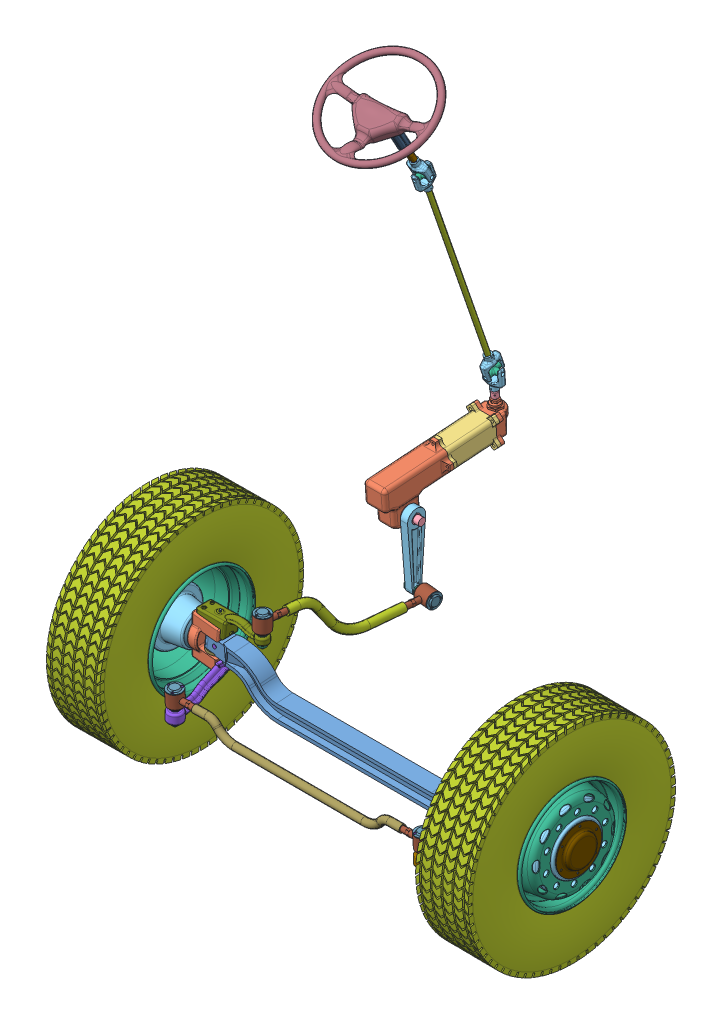
SolidWorks assembly ansamblu, configuration Default. Lengths in mm.
Overall size (2476.69 3208.04 2204.97).
90 component instances, 46 part files, 220 mates.
Components (placement in the parent):
- grinda-1: grinda [Default] at (1439.9442 78.9332 18.0501) x (0 -0.069756 0.997564) z (0 -0.997564 -0.069756) size (90 1677.81 247.94)
- stanga-1: stanga [Default] at (364.9939 177.7719 27.5856) x (0.999964 0.000299 -0.008501) z (0.008501 -0.000519 0.999964) size (496.03 235.4 150)
- stanga-2: stanga [Default] at (2514.8929 177.7718 27.7536) x (-0.999959 0.000299 -0.009102) z (0.009102 0.000592 -0.999958) size (496.03 235.4 150)
- pivot-1: pivot [Default] at (2221.7799 289.9237 25.1519) x (0.121572 -0.992582 0.000519) z (0.992546 0.121572 0.008501) size (225 64 64)
- pivot-2: pivot [Default] at (658.1085 289.9237 25.1519) x (-0.121572 -0.992582 0.000519) z (-0.992546 0.121572 0.008501) size (225 64 64)
- flansa-1: flansa [Default] at (640.7236 147.9844 25.2261) x (-0.233057 0.029053 0.972029) z (0.964834 -0.118051 0.23486) size (85 15 85)
- flansa-2: flansa [Default] at (2240.9883 133.0957 25.2339) x (-0.59496 -0.072453 0.800483) z (-0.794508 -0.097625 -0.599355) size (85 15 85)
- suport roata-1: suport roata [Default] at (2627.8883 177.738 28.7822) x (-0.999959 0.000299 -0.009102) z (-0.009075 0.051421 0.998636) size (310 410 410)
- janta-1: janta [Default] at (2627.8883 177.738 28.7822) x (-0.999959 0.000299 -0.009102) z (-0.007793 -0.545407 0.838135) size (329.22 591.5 591.5)
- janta-2: janta [Default] at (251.998 177.7381 28.5463) x (0.999964 0.000299 -0.008501) z (-0.008163 -0.247389 -0.968882) size (329.22 591.5 591.5)
- suport roata-2: suport roata [Default] at (251.998 177.7381 28.5463) x (0.999964 0.000299 -0.008501) z (0.008163 0.247389 0.968882) size (310 410 410)
- anvelopa-1: anvelopa [Default] at (2462.5448 177.7875 27.2771) x (0.999959 -0.000299 0.009102) z (0.004518 0.884121 -0.467236) size (314.46 1137.72 1137.72)
- anvelopa-2: anvelopa [Default] at (417.3423 177.7876 27.1406) x (-0.999964 -0.000299 0.008501) z (-0.007971 0.381904 -0.924168) size (314.46 1137.72 1137.72)
- dreapta-1: dreapta [Default] at (688.4721 88.533 31.2896) x (-0.008501 0.000519 -0.999964) z (0.999964 0.000299 -0.008501) size (420.57 104.39 147.63)
- stg-1: stg [Default] at (2285.6306 88.5031 34.1142) x (0.009102 0.000592 -0.999958) z (0.999959 -0.000299 0.009102) size (420.57 104.39 109.31)
- bila-1: bila [Default] at (751.0425 -9.2105 363.8556) x (0.011469 0.999933 -0.001733) z (-0.070514 0.002537 0.997508) size (149.01 50 50)
- bila-2: bila [Default] at (2128.6242 -9.2366 365.7775) x (-0.011468 0.999933 -0.001666) z (-0.141589 0.000026 0.989926) size (149.01 50 50)
- art1-1: art1 [Default] at (752.467 86.0292 361.6292) x (-0.000079 0.997564 0.069756) z (-0.001402 -0.069756 0.997563) size (83 220.5 80.5)
- art1-2: art1 [Default] at (2127.2043 86.0031 363.5595) x (-0.000079 0.997564 0.069756) z (0.001402 0.069756 -0.997563) size (83 220.5 80.5)
- bara-1: bara [Default] at (862.7136 127.8222 364.7066) x (0.999999 -0.000019 0.001404) z (-0.001402 -0.069756 0.997563) size (1150 115 40)
- bucsa art1-1: bucsa art1 [Default] at (752.4647 114.7941 363.6407) x (-0.143093 -0.06905 0.987298) z (-0.989709 0.009904 -0.14275) size (50.5 28 50.5)
- bucsa art1-2: bucsa art1 [Default] at (2127.202 114.7679 365.5709) x (-0.143093 -0.06905 0.987298) z (-0.989709 0.009904 -0.14275) size (50.5 28 50.5)
- capac art1-1: capac art1 [Default] at (752.46 174.6479 367.8261) x (-0.866726 -0.034862 0.497566) z (-0.498785 0.06042 -0.864617) size (80.5 11 80.5)
- arc art1-1: arc art1 [Default] at (752.46 174.6479 367.8261) x (-0.269709 -0.067193 0.960595) z (0.000079 -0.997564 -0.069756) size (37.4 37.4 27.2)
- arc art1-2: arc art1 [Default] at (2127.1972 174.6218 369.7563) x (-0.131958 -0.069157 0.98884) z (0.000079 -0.997564 -0.069756) size (37.4 37.4 27.2)
- capac art1-2: capac art1 [Default] at (2127.1972 174.6218 369.7563) x (-0.001402 -0.069756 0.997563) z (-0.999999 0.000019 -0.001404) size (80.5 11 80.5)
- princ-1: princ [Default] at (706.7666 278.9042 -17.769) x (0.999964 0.000299 -0.008501) z (0.008501 -0.000519 0.999964) size (358.77 112.91 85)
- surub-1: surub [Default] at (720.4615 155.6948 366.4558) x (-0.679245 0.051141 -0.732127) z (-0.000079 0.997564 0.069756) size (12 12 21.92)
- surub-2: surub [Default] at (768.5003 157.627 338.8779) x (-0.54809 0.058302 -0.834385) z (-0.000079 0.997564 0.069756) size (12 12 21.92)
- surub-3: surub [Default] at (768.4226 153.7607 394.1684) x (0.724056 0.048171 -0.688057) z (-0.000079 0.997564 0.069756) size (12 12 21.92)
- surub-4: surub [Default] at (2111.2376 157.6015 340.7632) x (0.811695 0.040807 -0.582655) z (-0.000079 0.997564 0.069756) size (12 12 21.92)
- surub-5: surub [Default] at (2159.1987 155.6675 368.4758) x (0.827533 -0.039097 0.560054) z (-0.000079 0.997564 0.069756) size (12 12 21.92)
- surub-6: surub [Default] at (2111.1599 153.7352 396.0537) x (-0.989084 0.010201 -0.147) z (-0.000079 0.997564 0.069756) size (12 12 21.92)
- rul1-1: rul1 [Default] at (301.9962 177.7531 28.1212) x (0.999964 0.000299 -0.008501) z (0.008306 -0.249815 0.968258) size (30 100 100)
- rul1-2: rul1 [Default] at (2577.8903 177.753 28.3271) x (-0.999959 0.000299 -0.009102) z (0.003112 -0.928053 -0.372436) size (30 100 100)
- rul2-1: rul2 [Default] at (2369.899 177.8152 26.4338) x (0.999959 -0.000299 0.009102) z (0.007754 -0.496245 -0.868148) size (32 140 140)
- rul2-2: rul2 [Default] at (509.9887 177.8153 26.353) x (-0.999964 -0.000299 0.008501) z (-0.006732 0.638726 -0.769405) size (32 140 140)
- caseta 1-1: caseta 1 [Default] at (751.51 430.3169 -690.1638) x (0 0.069756 -0.997564) z (1 0 0) size (350 280 180)
- caseta 2-1: caseta 2 [Default] at (811.51 637.9487 -1166.8413) x (0 0.069756 -0.997564) z (1 0 0) size (267 180 180)
- caseta3-1: caseta3 [Default] at (831.51 472.3435 -812.5303) x (1 0 0) z (0 -0.006931 0.999976) size (110 80 80)
- caseta 4-1: caseta 4 [Default] at (891.51 472.3435 -812.5303) x (0 -0.999976 -0.006931) z (1 0 0) size (415 100 42.07)
- bila 2-1: bila 2 [Default] at (894.4397 265.9382 23.1303) x (-0.000295 1 0.000521) z (-0.100733 -0.000548 0.994913) size (133.91 50 50)
- bila 2-2: bila 2 [Default] at (848.51 132.3517 -814.8869) x (1 0 0) z (0 0.967081 -0.254469) size (133.91 50 50)
- art1-3: art1 [Default] at (894.2202 346.0165 23.1921) x (0.0065 0.999979 -0.000175) z (0.995708 -0.006456 0.092322) size (83 220.5 80.5)
- art1-4: art1 [Default] at (928.7116 132.5378 -817.549) x (0.995708 -0.006456 0.092322) z (0.0065 0.999979 -0.000175) size (83 220.5 80.5)
- bara 2-1: bara 2 [Default] at (905.5938 387.8197 -96.5517) x (0.092319 -0.000774 -0.995729) z (0.995708 -0.006456 0.092322) size (600 300 45)
- capac art1-3: capac art1 [Default] at (894.7976 434.8497 23.1766) x (0.417904 -0.002557 0.908488) z (-0.908468 0.005978 0.417912) size (80.5 11 80.5)
- capac art1-4: capac art1 [Default] at (1017.1654 131.9643 -809.3476) x (-0.0065 -0.999979 0.000175) z (-0.092319 0.000774 0.995729) size (80.5 11 80.5)
- arc art1-3: arc art1 [Default] at (1017.1654 131.9643 -809.3476) x (0.074625 -0.53399 -0.842191) z (-0.995708 0.006456 -0.092322) size (37.4 37.4 27.2)
- arc art1-4: arc art1 [Default] at (894.7976 434.8497 23.1766) x (-0.090246 0.000761 0.995919) z (-0.0065 -0.999979 0.000175) size (37.4 37.4 27.2)
- bucsa art1-3: bucsa art1 [Default] at (894.4076 374.851 23.1871) x (-0.090246 0.000761 0.995919) z (-0.995898 0.006457 -0.090249) size (50.5 28 50.5)
- bucsa art1-4: bucsa art1 [Default] at (957.4229 132.3517 -814.8869) x (-0.092207 0.016216 0.995608) z (0.007924 0.999848 -0.015551) size (50.5 28 50.5)
- bolt-1: bolt [Default] at (672.7576 182.3215 -19.3828) x (0.008501 -0.000519 0.999964) z (-0.341315 -0.939946 0.002414) size (89 24 24)
- bucsa-1: bucsa [Default] at (657.5006 284.9608 25.1545) x (-0.121572 -0.992582 0.000519) z (0.065879 -0.00859 -0.997791) size (65 69 69)
- bucsa-2: bucsa [Default] at (638.7784 132.1031 25.2344) x (-0.121572 -0.992582 0.000519) z (0.065879 -0.00859 -0.997791) size (65 69 69)
- bolt-2: bolt [Default] at (2207.1308 182.3215 -19.3828) x (-0.008501 -0.000519 0.999964) z (-0.097193 -0.995265 -0.001343) size (89 24 24)
- bucsa-3: bucsa [Default] at (2241.1099 132.1031 25.2344) x (0.121572 -0.992582 0.000519) z (-0.596218 -0.073443 -0.799456) size (65 69 69)
- bucsa-4: bucsa [Default] at (2222.3878 284.9608 25.1545) x (0.121572 -0.992582 0.000519) z (0.157693 0.018798 -0.987309) size (65 69 69)
- capac 2-1: capac 2 [Default] at (2301.4269 294.6629 65.8814) x (0.009102 0.000592 -0.999958) z (0.992541 0.121572 0.009107) size (80 50 140)
- capac 3-1: capac 3 [Default] at (2249.5227 63.4164 25.2703) x (-0.121572 0.992582 -0.000519) z (0.009102 0.000592 -0.999958) size (6.2 104 80)
- capac 3-2: capac 3 [Default] at (630.3656 63.4164 25.2703) x (0.121572 0.992582 -0.000519) z (0.008501 -0.000519 0.999964) size (6.2 104 80)
- capacrul-1: capacrul [Default] at (2239.0432 148.977 25.2256) x (0.121572 -0.992582 0.000519) z (0.157693 0.018798 -0.987309) size (17 90.6 90.6)
- capacrul-2: capacrul [Default] at (640.8452 148.977 25.2256) x (-0.121572 -0.992582 0.000519) z (0.065879 -0.00859 -0.997791) size (17 90.6 90.6)
- volan1-1: volan1 [Default] at (811.51 2396.2001 -734.1632) x (0.998571 0.025911 -0.046745) z (0.053447 -0.484117 0.87337) size (555 121.31 555)
- Part1-1: Part1 [Default] at (546.9873 177.8264 26.0385) x (0.003216 -0.938494 0.345282) z (-0.999964 -0.000299 0.008501) size (160 160 10)
- Part1-2: Part1 [Default] at (2332.9005 177.8263 26.097) x (-0.004847 -0.86363 0.504103) z (0.999959 -0.000299 0.009102) size (160 160 10)
- flans-1: flans [Default] at (256.9978 177.7396 28.5038) x (0.999964 0.000299 -0.008501) z (0.008366 0.146468 0.98918) size (15 75 75)
- piulit-1: piulit [Default] at (256.9978 177.7396 28.5038) x (0.008501 -0.000519 0.999964) z (-0.999964 -0.000299 0.008501) size (70 80.83 40.09)
- siguranta-1: siguranta [Default] at (224.999 177.7301 28.7758) x (0.008501 -0.000519 0.999964) z (0.000295 -1 -0.000521) size (68.93 3 40.42)
- flans-2: flans [Default] at (2622.8885 177.7395 28.7367) x (-0.999959 0.000299 -0.009102) z (-0.008522 0.321675 0.946812) size (15 75 75)
- piulit-2: piulit [Default] at (2623.3884 177.7393 28.7412) x (-0.009102 -0.000592 0.999958) z (0.999959 -0.000299 0.009102) size (70 80.83 40.09)
- siguranta-2: siguranta [Default] at (2654.8871 177.7299 29.0279) x (-0.009102 -0.000592 0.999958) z (-0.000294 -1 -0.000595) size (68.93 3 40.42)
- capca-1: capca [Default] at (2672.8864 177.7245 29.1918) x (-0.999959 0.000299 -0.009102) z (0.003873 -0.89059 -0.45479) size (29 250 250)
- capca-2: capca [Default] at (206.9996 177.7247 28.9288) x (0.999964 0.000299 -0.008501) z (-0.008263 -0.203197 -0.979103) size (29 250 250)
- arur-1: arur [Default] at (661.6114 318.5236 25.137) x (-0.022311 0.003255 0.999746) z (-0.992332 0.12153 -0.022541) size (11.55 18.87 10)
- arur-2: arur [Default] at (2221.7799 289.9237 25.1519) x (-0.334278 -0.040451 0.941606) z (-0.934601 -0.114647 -0.336716) size (11.55 18.87 10)
- clt-1: clt [Default] at (811.51 631.8444 -1294.5783) x (-1 0 0) z (0 0.069756 -0.997564) size (163.64 181.82 107.5)
- cas-1: cas [Default] at (811.51 700.8714 -1349.898) x (0 0.997564 0.069756) z (-0.966481 0.017909 -0.256111) size (70 25 25)
- cupl-1: cupl [Default] at (811.51 809.6059 -1342.2945) x (-0.054488 0.069653 -0.996082) z (0 -0.997564 -0.069756) size (36 36 68)
- cruc-1: cruc [Default] at (811.51 830.5547 -1340.8296) x (-0.998514 -0.003801 0.054356) z (0 -0.997564 -0.069756) size (100 55 115)
- cruc-2: cruc [Default] at (811.51 2055.0984 -923.239) x (-0.998571 -0.025911 0.046745) z (0 0.87462 0.48481) size (100 55 115)
- cruc-3: cruc [Default] at (811.51 1973.1922 -959.706) x (0.052637 -0.325117 0.944208) z (0 -0.945519 -0.325568) size (100 55 115)
- cruc-4: cruc [Default] at (811.51 917.9935 -1323.04) x (0.052637 -0.325117 0.944208) z (0 0.945519 0.325568) size (100 55 115)
- cruc2-1: cruc2 [Default] at (811.51 2015.7405 -945.0554) x (0.009268 -0.945319 -0.326016) z (0.998571 0.025911 -0.046745) size (37 70 70)
- cruc2-2: cruc2 [Default] at (811.51 875.4451 -1337.6906) x (-0.014083 -0.945666 -0.324834) z (-0.998514 -0.003801 0.054356) size (37 70 70)
- bar1-1: bar1 [Default] at (811.51 937.8493 -1316.2031) x (0.052637 -0.325117 0.944208) z (0 0.945519 0.325568) size (30 30 1074)
- tja-1: tja [Default] at (811.51 2073.4654 -913.058) x (0.053447 -0.484117 0.87337) z (0 0.87462 0.48481) size (30 30 55)
- tja-2: tja [Default] at (811.51 2395.3255 -734.648) x (0.053447 -0.484117 0.87337) z (0 -0.87462 -0.48481) size (30 30 55)
- regl-1: regl [Default] at (811.5367 2107.3335 -893.7137) x (-0.053447 0.484117 -0.87337) z (0 0.87462 0.48481) size (39.27 39.27 190)
- regl2-1: regl2 [Default] at (811.5367 2299.7499 -787.0556) x (0.053447 -0.484117 0.87337) z (0 0.87462 0.48481) size (49.29 49.27 190)
Mates (geometry in assembly coordinates):
- Concentric1: concentric anti-aligned: cylinder of stanga-1 through (624.1141 12.3757 25.297) axis (0.121572 0.992582 -0.000519) radius 28; circle of grinda-1
- Coincident1: coincident anti-aligned: plane of stanga-1 through (616.3764 224.4795 -37.1015) normal (-0.121572 -0.992582 0.000519); plane of grinda-1 through (610.2565 225.2839 67.8696) normal (0.121572 0.992582 -0.000519)
- Coincident2: coincident aligned: circle of grinda-1; cylinder of stanga-2 through (2255.7743 12.3757 25.297) axis (-0.121572 0.992582 -0.000519) radius 28
- Coincident3: coincident anti-aligned: plane of grinda-1 through (2269.6318 225.2839 67.8696) normal (-0.121572 0.992582 -0.000519); plane of stanga-2 through (2259.7441 224.0841 89.3692) normal (0.121572 -0.992582 0.000519)
- Concentric3: concentric aligned: cylinder of stanga-2 through (2255.7743 12.3757 25.297) axis (-0.121572 0.992582 -0.000519) radius 28; cylinder of pivot-1 through (2221.7799 289.9237 25.1519) axis (-0.121572 0.992582 -0.000519) radius 26
- Coincident5: coincident anti-aligned: plane of stanga-2 through (2158.681 277.1734 54.8328) normal (-0.121572 0.992582 -0.000519); plane of pivot-1 through (2222.6598 284.9774 -6.8443) normal (0.121572 -0.992582 0.000519)
- Concentric4: concentric aligned: cylinder of stanga-1 through (624.1141 12.3757 25.297) axis (0.121572 0.992582 -0.000519) radius 28; cylinder of pivot-2 through (658.1085 289.9237 25.1519) axis (0.121572 0.992582 -0.000519) radius 26
- Coincident6: coincident anti-aligned: plane of stanga-1 through (719.3262 277.3709 -8.3118) normal (0.121572 0.992582 -0.000519); plane of pivot-2 through (657.7726 284.9442 57.1533) normal (-0.121572 -0.992582 0.000519)
- Concentric5: concentric aligned: cylinder of pivot-1 through (2221.7799 289.9237 25.1519) axis (-0.121572 0.992582 -0.000519) radius 26; cylinder of flansa-2 through (2236.5446 169.3769 25.2149) axis (-0.121572 0.992582 -0.000519) radius 27.5
- Concentric6: concentric anti-aligned: cylinder of pivot-2 through (658.1085 289.9237 25.1519) axis (0.121572 0.992582 -0.000519) radius 26; cylinder of flansa-1 through (636.2798 111.7033 25.245) axis (-0.121572 -0.992582 0.000519) radius 27.5
- Concentric7: concentric aligned: cylinder of stanga-2 through (2563.3347 175.227 144.7309) axis (0.939481 -0.007533 0.342518) radius 30; cylinder of suport roata-1 through (2644.0504 174.5799 174.1584) axis (0.939481 -0.007533 0.342518) radius 60
- Concentric8: concentric aligned: cylinder of suport roata-1 through (2644.0504 174.5799 174.1584) axis (0.939481 -0.007533 0.342518) radius 140; circle of janta-1
- Coincident14: coincident anti-aligned: plane of suport roata-1 through (2599.0032 -29.8089 169.2484) normal (0.939481 -0.007533 0.342518); plane of janta-1 through (2629.5164 57.037 87.4647) normal (-0.939481 0.007533 -0.342518)
- Concentric9: concentric aligned: cylinder of suport roata-1 through (2335.9176 344.3461 52.4114) axis (0.939481 -0.007533 0.342518) radius 15; circle of janta-1
- Concentric10: concentric anti-aligned: circle of janta-2; circle of suport roata-2
- Concentric11: concentric aligned: circle of janta-2; circle of suport roata-2
- Coincident15: coincident anti-aligned: plane of janta-2 through (259.2024 39.5096 -53.6164) normal (0.958207 0.005567 0.286022); plane of suport roata-2 through (281.7791 374.3403 -135.7686) normal (-0.958207 -0.005567 -0.286022)
- Concentric12: concentric aligned: cylinder of stanga-1 through (310.0194 175.9128 -74.5959) axis (-0.958207 -0.005567 -0.286022) radius 45; cylinder of suport roata-2 through (227.6948 175.4344 -99.1696) axis (-0.958207 -0.005567 -0.286022) radius 60
- Coincident16: coincident anti-aligned: plane of stanga-1 through (546.4808 222.2563 -5.6816) normal (-0.958207 -0.005567 -0.286022); plane of suport roata-2 through (550.8375 245.1237 -20.7222) normal (0.958207 0.005567 0.286022)
- Distance1: distance = 63.34 mm anti-aligned: plane of anvelopa-2 through (531.9472 436.4134 133.0268) normal (-0.999964 -0.000299 0.008501); plane of janta-2 through (468.3898 -69.7565 89.9171) normal (0.999964 0.000299 -0.008501)
- Concentric13: concentric anti-aligned: cylinder of janta-2 through (230.7586 175.4522 -98.255) axis (-0.958207 -0.005567 -0.286022) radius 279.7426; cylinder of anvelopa-2 through (469.6481 176.8402 -26.9472) axis (0.958207 0.005567 0.286022) radius 279.8
- Distance2: distance = 63.34 mm anti-aligned: plane of anvelopa-1 through (2350.9842 47.0828 -221.1257) normal (0.999959 -0.000299 0.009102); plane of janta-1 through (2413.3133 -36.351 -112.529) normal (-0.999959 0.000299 -0.009102)
- Concentric14: concentric anti-aligned: cylinder of janta-1 through (2641.0465 174.604 173.0632) axis (0.939481 -0.007533 0.342518) radius 279.7426; cylinder of anvelopa-1 through (2406.8255 176.4819 87.6705) axis (-0.939481 0.007533 -0.342518) radius 279.8
- Coincident21: coincident anti-aligned: plane of stanga-1 through (700.2875 59.0674 -5.8978) normal (0.958207 0.005567 0.286022); plane of dreapta-1 through (684.2618 89.057 47.2064) normal (-0.958207 -0.005567 -0.286022)
- Coincident26: coincident anti-aligned: plane of stanga-2 through (2177.8702 58.8858 52.1928) normal (-0.939481 0.007533 -0.342518); plane of stg-1 through (2191.8853 88.5816 14.4041) normal (0.939481 -0.007533 0.342518)
- Concentric15: concentric aligned: cylinder of stanga-1 through (676.2281 70.8129 11.5432) axis (0.958207 0.005567 0.286022) radius 6.5; cylinder of dreapta-1 through (683.5183 70.8553 13.7193) axis (0.958207 0.005567 0.286022) radius 5
- Concentric18: concentric aligned: cylinder of stanga-1 through (661.9263 72.5896 59.4212) axis (0.958207 0.005567 0.286022) radius 6.5; cylinder of dreapta-1 through (669.2165 72.632 61.5973) axis (0.958207 0.005567 0.286022) radius 5
- Concentric19: concentric anti-aligned: cylinder of stanga-2 through (2220.0493 72.8087 -10.6409) axis (-0.939481 0.007533 -0.342518) radius 6.5; circle of stg-1
- Concentric20: concentric anti-aligned: circle of stanga-2; circle of stg-1
- Concentric21: concentric aligned: cylinder of dreapta-1 through (647.0231 81.6449 384.0838) axis (-0.016738 -0.99927 0.034332) radius 10; cylinder of bila-1 through (645.7176 3.7018 386.7617) axis (-0.016738 -0.99927 0.034332) radius 10
- Coincident29: coincident anti-aligned: plane of dreapta-1 through (646.1025 26.685 385.9721) normal (-0.016738 -0.99927 0.034332); plane of bila-1 through (626.1545 26.9706 384.5602) normal (0.016738 0.99927 -0.034332)
- Coincident30: coincident anti-aligned: circle of stg-1; cylinder of bila-2 through (2022.3751 -22.2831 302.5782) axis (0.017463 -0.999218 -0.035473) radius 10
- Coincident31: coincident anti-aligned: plane of stg-1 through (2021.9735 0.6989 303.394) normal (0.017463 -0.999218 -0.035473); plane of bila-2 through (2002.1765 0.4534 300.5622) normal (-0.017463 0.999218 0.035473)
- Concentric22: concentric: sphere of bila-1; sphere of art1-1
- Concentric23: concentric: sphere of bila-2; sphere of art1-2
- Parallel12: parallel anti-aligned: plane of art1-1 through (828.0348 137.2443 373.4965) normal (0.998311 -0.018906 -0.054939); plane of art1-2 through (1840.56 118.0686 317.7751) normal (-0.998311 0.018906 0.054939)
- Parallel13: parallel aligned: cylinder of art1-1 through (647.7933 127.6242 382.5041) axis (0.02266 0.997392 0.068527) radius 25.25; cylinder of art1-2 through (2020.2095 101.6328 306.9773) axis (0.02266 0.997392 0.068527) radius 25.25
- Concentric30: concentric anti-aligned: cylinder of art1-1 through (828.0348 137.2443 373.4965) axis (-0.998311 0.018906 0.054939) radius 15; cylinder of art1-2 through (1840.56 118.0686 317.7751) axis (0.998311 -0.018906 -0.054939) radius 15
- Distance7: distance = 1294.2386 mm: cylinder of art1-1 through (752.4647 114.7941 363.6407) axis (-0.000079 0.997564 0.069756) radius 40.25; cylinder of art1-2 through (2127.202 114.7679 365.5709) axis (-0.000079 0.997564 0.069756) radius 40.25
- Concentric32: concentric anti-aligned: cylinder of art1-1 through (828.0348 137.2443 373.4965) axis (-0.998311 0.018906 0.054939) radius 15; cylinder of bara-1 through (1835.6936 118.1608 318.043) axis (0.998311 -0.018906 -0.054939) radius 15
- Distance8: distance = 25 mm anti-aligned: plane of bara-1 through (862.7136 127.8222 364.7066) normal (-0.999999 0.000019 -0.001404); plane of art1-1 through (837.7169 86.0276 361.7489) normal (0.999999 -0.000019 0.001404)
- Concentric33: concentric aligned: cylinder of art1-1 through (647.7933 127.6242 382.5041) axis (0.02266 0.997392 0.068527) radius 25.25; cylinder of bucsa art1-1 through (650.243 235.4485 389.9124) axis (0.02266 0.997392 0.068527) radius 25.25
- Concentric34: concentric: sphere of bila-1; sphere of bucsa art1-1
- Concentric35: concentric aligned: cylinder of art1-2 through (2020.2095 101.6328 306.9773) axis (0.02266 0.997392 0.068527) radius 25.25; cylinder of bucsa art1-2 through (2022.6592 209.457 314.3855) axis (0.02266 0.997392 0.068527) radius 25.25
- Concentric36: concentric: sphere of bila-2; sphere of bucsa art1-2
- Coincident32: coincident anti-aligned: plane of art1-1 through (608.8123 181.2469 388.3474) normal (0.02266 0.997392 0.068527); plane of capac art1-1 through (682.7162 181.2288 364.1738) normal (-0.02266 -0.997392 -0.068527)
- Concentric37: concentric aligned: circle of art1-1; circle of capac art1-1
- Concentric38: concentric aligned: cylinder of art1-1 through (616.5951 161.1431 386.5236) axis (0.02266 0.997392 0.068527) radius 4; cylinder of capac art1-1 through (617.0483 181.091 387.8941) axis (0.02266 0.997392 0.068527) radius 4
- Coincident34: coincident anti-aligned: plane of capac art1-1 through (666.8528 187.8576 375.0883) normal (-0.02266 -0.997392 -0.068527); plane of arc art1-1 through (672.5997 187.9246 372.2125) normal (0.02266 0.997392 0.068527)
- Coincident35: coincident anti-aligned: plane of bucsa art1-1 through (652.1982 164.1642 359.9655) normal (0.02266 0.997392 0.068527); plane of arc art1-1 through (671.9469 162.9706 370.807) normal (-0.02266 -0.997392 -0.068527)
- Coincident38: coincident: axis of art1-1 through (647.3115 106.4179 381.0471) axis (0.02266 0.997392 0.068527); point of arc art1-1
- Coincident39: coincident anti-aligned: plane of bucsa art1-2 through (2024.6145 138.1728 284.4387) normal (0.02266 0.997392 0.068527); plane of arc art1-2 through (2042.1557 137.2443 292.1524) normal (-0.02266 -0.997392 -0.068527)
- Coincident40: coincident: axis of art1-2 through (2019.7277 80.4264 305.5203) axis (0.02266 0.997392 0.068527); point of arc art1-2
- Coincident41: coincident anti-aligned: plane of art1-2 through (2061.5925 153.7336 308.3979) normal (0.02266 0.997392 0.068527); plane of capac art1-2 through (2019.2571 157.2982 270.5148) normal (-0.02266 -0.997392 -0.068527)
- Coincident42: coincident aligned: cylinder of art1-2 through (2020.2095 101.6328 306.9773) axis (0.02266 0.997392 0.068527) radius 40.25; circle of capac art1-2
- Concentric39: concentric aligned: cylinder of art1-2 through (2052.9033 133.9417 307.4806) axis (0.02266 0.997392 0.068527) radius 4; cylinder of capac art1-2 through (2053.3565 153.8895 308.8512) axis (0.02266 0.997392 0.068527) radius 4
- Coincident43: coincident anti-aligned: plane of stanga-1 through (711.4239 212.853 -8.2781) normal (0.950476 -0.116265 0.288234); plane of princ-1 through (692.8679 280.6578 80.2625) normal (-0.950476 0.116265 -0.288234)
- Coincident44: coincident anti-aligned: plane of stanga-1 through (719.3262 277.3709 -8.3118) normal (0.121572 0.992582 -0.000519); plane of princ-1 through (692.8679 280.6578 80.2625) normal (-0.121572 -0.992582 0.000519)
- Concentric40: concentric anti-aligned: cylinder of stanga-1 through (682.6108 253.6806 33.816) axis (0.950476 -0.116265 0.288234) radius 6.5; cylinder of princ-1 through (730.6757 247.8011 48.3918) axis (-0.950476 0.116265 -0.288234) radius 7
- Coincident45: coincident aligned: cylinder of art1-1 through (616.5951 161.1431 386.5236) axis (0.02266 0.997392 0.068527) radius 4; circle of surub-1
- Coincident46: coincident anti-aligned: plane of capac art1-1 through (617.1163 184.0831 388.0997) normal (0.02266 0.997392 0.068527); plane of surub-1 through (617.1163 184.0831 388.0997) normal (-0.02266 -0.997392 -0.068527)
- Coincident47: coincident anti-aligned: plane of capac art1-1 through (663.5526 185.106 357.8569) normal (0.02266 0.997392 0.068527); plane of surub-2 through (663.5526 185.106 357.8569) normal (-0.02266 -0.997392 -0.068527)
- Concentric41: concentric anti-aligned: cylinder of art1-1 through (663.0314 162.166 356.2808) axis (0.02266 0.997392 0.068527) radius 4; cylinder of surub-2 through (663.5526 185.106 357.8569) axis (-0.02266 -0.997392 -0.068527) radius 4
- Coincident48: coincident aligned: plane of capac art1-1 through (666.5179 181.2453 413.0684) normal (0.02266 0.997392 0.068527); circle of surub-3
- Concentric42: concentric anti-aligned: cylinder of art1-1 through (665.9967 158.3052 411.4922) axis (0.02266 0.997392 0.068527) radius 4; cylinder of surub-3 through (666.5179 181.2453 413.0684) axis (-0.02266 -0.997392 -0.068527) radius 4
- Coincident49: coincident anti-aligned: plane of capac art1-2 through (2004.0229 159.7196 284.0881) normal (0.02266 0.997392 0.068527); plane of surub-4 through (2004.0229 159.7196 284.0881) normal (-0.02266 -0.997392 -0.068527)
- Coincident50: coincident aligned: circle of capac art1-2; cylinder of surub-4 through (2004.0229 159.7196 284.0881) axis (-0.02266 -0.997392 -0.068527) radius 4
- Coincident51: coincident anti-aligned: plane of capac art1-2 through (2053.4245 156.8817 309.0568) normal (0.02266 0.997392 0.068527); plane of surub-5 through (2053.4245 156.8817 309.0568) normal (-0.02266 -0.997392 -0.068527)
- Coincident52: coincident aligned: circle of capac art1-2; cylinder of surub-5 through (2053.4245 156.8817 309.0568) axis (-0.02266 -0.997392 -0.068527) radius 4
- Coincident53: coincident anti-aligned: plane of capac art1-2 through (2006.9882 155.8588 339.2995) normal (0.02266 0.997392 0.068527); plane of surub-6 through (2006.9882 155.8588 339.2995) normal (-0.02266 -0.997392 -0.068527)
- Concentric43: concentric anti-aligned: cylinder of art1-2 through (2006.467 132.9188 337.7234) axis (0.02266 0.997392 0.068527) radius 4; cylinder of surub-6 through (2006.9882 155.8588 339.2995) axis (-0.02266 -0.997392 -0.068527) radius 4
- Coincident54: coincident anti-aligned: plane of stanga-2 through (2331.3866 222.0442 62.1528) normal (0.939481 -0.007533 0.342518); plane of suport roata-1 through (2329.9477 107.1837 63.5736) normal (-0.939481 0.007533 -0.342518)
- Concentric45: concentric aligned: cylinder of suport roata-2 through (227.6948 175.4344 -99.1696) axis (-0.958207 -0.005567 -0.286022) radius 50; cylinder of rul1-1 through (316.2937 175.9492 -72.723) axis (-0.958207 -0.005567 -0.286022) radius 50
- Coincident55: coincident anti-aligned: plane of suport roata-2 through (319.561 224.4052 -84.6119) normal (-0.958207 -0.005567 -0.286022); plane of rul1-1 through (312.6043 222.416 -61.2676) normal (0.958207 0.005567 0.286022)
- Concentric46: concentric aligned: cylinder of stanga-2 through (2563.3347 175.227 144.7309) axis (0.939481 -0.007533 0.342518) radius 30; cylinder of rul1-2 through (2557.183 175.2764 142.4881) axis (0.939481 -0.007533 0.342518) radius 30
- Coincident56: coincident aligned: plane of stanga-2 through (2585.1891 200.0282 153.802) normal (0.939481 -0.007533 0.342518); plane of rul1-2 through (2595.6292 186.9284 124.878) normal (0.939481 -0.007533 0.342518)
- Coincident57: coincident anti-aligned: plane of suport roata-1 through (2360.011 106.9426 74.5341) normal (-0.939481 0.007533 -0.342518); plane of rul2-1 through (2349.7677 117.8539 102.8702) normal (0.939481 -0.007533 0.342518)
- Concentric47: concentric anti-aligned: cylinder of rul2-1 through (2361.7709 176.8431 71.2444) axis (-0.939481 0.007533 -0.342518) radius 45; cylinder of stanga-2 through (2563.3347 175.227 144.7309) axis (0.939481 -0.007533 0.342518) radius 45
- Coincident58: coincident anti-aligned: plane of suport roata-2 through (520.1749 244.9456 -29.8749) normal (0.958207 0.005567 0.286022); plane of rul2-2 through (502.8855 229.3896 28.3493) normal (-0.958207 -0.005567 -0.286022)
- Concentric48: concentric anti-aligned: circle of rul1-1; circle of rul2-2
- Coincident59: coincident anti-aligned: plane of caseta 1-1 through (871.51 673.0732 -1024.0433) normal (0 0.069756 -0.997564); plane of caseta 2-1 through (811.51 661.1025 -1024.8804) normal (0 -0.069756 0.997564)
- Concentric49: concentric anti-aligned: cylinder of caseta 1-1 through (811.51 608.3364 -958.3992) axis (0 0.069756 -0.997564) radius 48; cylinder of caseta 2-1 through (811.51 611.0048 -996.5581) axis (0 -0.069756 0.997564) radius 48
- Concentric50: concentric anti-aligned: cylinder of caseta 1-1 through (735.51 608.3364 -958.3992) axis (0 0.069756 -0.997564) radius 6; cylinder of caseta 2-1 through (735.51 622.9853 -1167.8877) axis (0 -0.069756 0.997564) radius 6
- Distance10: distance = 686 mm anti-aligned: plane of caseta 1-1 through (871.51 648.6585 -674.8959) normal (0 -0.069756 0.997564); plane of grinda-1 through (1812.0592 82.0722 -26.8403) normal (0 0.069756 -0.997564)
- Distance11: distance = 400 mm anti-aligned: plane of caseta 1-1 through (871.51 542.9021 -882.7795) normal (0 -0.997564 -0.069756); plane of grinda-1 through (1812.0592 75.7941 62.9405) normal (0 0.997564 0.069756)
- Distance13: distance = 250 mm: plane of caseta 1-1 through (761.51 430.3169 -690.1638) normal (-1 0 0); line of grinda-1 through (1011.51 75.7941 62.9405) axis (0 0.069756 -0.997564)
- Concentric51: concentric anti-aligned: cylinder of caseta 1-1 through (787.51 472.3435 -812.5303) axis (1 0 0) radius 30; cylinder of caseta3-1 through (816.8252 472.3435 -812.5303) axis (-1 0 0) radius 30
- Coincident66: coincident anti-aligned: plane of caseta 1-1 through (861.51 430.3169 -690.1638) normal (1 0 0); plane of caseta3-1 through (861.51 501.8145 -818.1392) normal (-1 0 0)
- Coincident67: coincident anti-aligned: cylinder of caseta3-1 through (816.8252 472.3435 -812.5303) axis (-1 0 0) radius 25; circle of caseta 4-1
- Coincident68: coincident anti-aligned: plane of caseta3-1 through (871.51 511.6382 -820.0089) normal (1 0 0); plane of caseta 4-1 through (871.51 472.3435 -812.5303) normal (-1 0 0)
- Coincident69: coincident aligned: plane of caseta3-1 through (863.553 491.2077 -819.1744) normal (0 0.186966 0.982366); plane of caseta 4-1 through (870.4745 501.2536 -821.0863) normal (0 0.186966 0.982366)
- Parallel17: parallel anti-aligned: plane of grinda-1 through (1812.0592 59.8538 4.1854) normal (0 0.069756 -0.997564); plane of caseta 1-1 through (871.51 648.6585 -674.8959) normal (0 -0.069756 0.997564)
- Coincident70: coincident anti-aligned: circle of princ-1; cylinder of bila 2-1 through (884.4478 267.1988 93.6057) axis (-0.004832 -0.999353 0.035642) radius 10
- Coincident71: coincident anti-aligned: plane of princ-1 through (884.7523 330.158 91.3603) normal (0.004832 0.999353 -0.035642); plane of bila 2-1 through (874.8032 330.1702 90.3527) normal (-0.004832 -0.999353 0.035642)
- Concentric53: concentric aligned: cylinder of caseta 4-1 through (911.51 138.339 -748.9618) axis (-1 0 0) radius 10; cylinder of bila 2-2 through (848.51 138.339 -748.9618) axis (-1 0 0) radius 10
- Coincident72: coincident anti-aligned: plane of caseta 4-1 through (911.51 472.3435 -812.5303) normal (1 0 0); plane of bila 2-2 through (911.51 135.7943 -758.6326) normal (-1 0 0)
- Concentric54: concentric: sphere of bila 2-2; sphere of art1-4
- Concentric55: concentric: sphere of bila 2-1; sphere of art1-3
- Parallel18: parallel anti-aligned: plane of art1-3 through (903.7319 389.9888 -89.4807) normal (0.10358 0.004916 -0.994609); plane of art1-4 through (951.744 137.3583 -568.3311) normal (-0.10358 -0.004916 0.994609)
- Parallel19: parallel anti-aligned: cylinder of art1-3 through (903.7319 389.9888 -89.4807) axis (-0.10358 -0.004916 0.994609) radius 15; cylinder of art1-4 through (951.744 137.3583 -568.3311) axis (0.10358 0.004916 -0.994609) radius 15
- Concentric57: concentric aligned: cylinder of art1-4 through (951.744 137.3583 -568.3311) axis (0.10358 0.004916 -0.994609) radius 15; cylinder of bara 2-1 through (938.5973 136.7343 -442.093) axis (0.10358 0.004916 -0.994609) radius 15
- Concentric58: concentric aligned: cylinder of art1-3 through (903.7319 389.9888 -89.4807) axis (-0.10358 -0.004916 0.994609) radius 15; cylinder of bara 2-1 through (903.4763 389.9767 -87.026) axis (-0.10358 -0.004916 0.994609) radius 15
- Distance14: distance = 35 mm anti-aligned: plane of art1-4 through (920.8414 132.6039 -732.6631) normal (-0.092319 0.000774 0.995729); plane of bara 2-1 through (959.3276 132.3605 -693.9446) normal (0.092319 -0.000774 -0.995729)
- Distance15: distance = 35 mm anti-aligned: plane of bara 2-1 through (905.5938 387.8197 -96.5517) normal (-0.092319 0.000774 0.995729); plane of art1-3 through (902.0903 345.9505 -61.6938) normal (0.092319 -0.000774 -0.995729)
- Perpendicular1: perpendicular: cylinder of art1-3 through (884.9741 376.0412 89.7239) axis (0.006692 0.999962 0.005639) radius 40.25; cylinder of art1-4 through (957.4229 138.339 -748.9618) axis (0.994599 -0.00724 0.103544) radius 40.25
- Concentric59: concentric: sphere of bila 2-1; sphere of bucsa art1-3
- Concentric60: concentric aligned: cylinder of art1-3 through (884.9741 376.0412 89.7239) axis (0.006692 0.999962 0.005639) radius 25.25; cylinder of bucsa art1-3 through (885.6976 484.1433 90.3335) axis (0.006692 0.999962 0.005639) radius 25.25
- Coincident76: coincident anti-aligned: plane of capac art1-4 through (1017.2402 159.03 -742.6301) normal (-0.994599 0.00724 -0.103544); plane of arc art1-3 through (1016.5568 164.4976 -735.683) normal (0.994599 -0.00724 0.103544)
- Coincident77: coincident: axis of capac art1-4 through (1014.115 137.9262 -743.0598) axis (0.994599 -0.00724 0.103544); point of arc art1-3
- Coincident78: coincident anti-aligned: plane of capac art1-3 through (876.7647 436.2053 70.7712) normal (-0.006692 -0.999962 -0.005639); plane of arc art1-4 through (905.8219 436.006 71.6403) normal (0.006692 0.999962 0.005639)
- Coincident79: coincident: axis of capac art1-3 through (885.3288 429.0392 90.0227) axis (0.006692 0.999962 0.005639); point of arc art1-4
- Coincident80: coincident anti-aligned: plane of art1-3 through (881.1597 428.8413 130.0558) normal (0.006692 0.999962 0.005639); plane of capac art1-3 through (868.9231 429.3562 53.2693) normal (-0.006692 -0.999962 -0.005639)
- Coincident81: coincident aligned: cylinder of art1-3 through (884.9741 376.0412 89.7239) axis (0.006692 0.999962 0.005639) radius 40.25; circle of capac art1-3
- Concentric61: concentric anti-aligned: cylinder of art1-3 through (881.8804 408.8826 121.7374) axis (0.006692 0.999962 0.005639) radius 4; circle of capac art1-3
- Concentric62: concentric: sphere of bila 2-2; sphere of bucsa art1-4
- Concentric63: concentric aligned: cylinder of art1-4 through (957.4229 138.339 -748.9618) axis (0.994599 -0.00724 0.103544) radius 25.25; cylinder of bucsa art1-4 through (1064.9452 137.5562 -737.7681) axis (0.994599 -0.00724 0.103544) radius 25.25
- Coincident82: coincident anti-aligned: plane of art1-4 through (1014.3057 138.1531 -783.507) normal (0.994599 -0.00724 0.103544); plane of capac art1-4 through (1010.406 178.2037 -743.247) normal (-0.994599 0.00724 -0.103544)
- Coincident83: coincident aligned: cylinder of art1-4 through (957.4229 138.339 -748.9618) axis (0.994599 -0.00724 0.103544) radius 40.25; circle of capac art1-4
- Coincident84: coincident anti-aligned: cylinder of art1-4 through (988.7728 165.7331 -729.4748) axis (0.994599 -0.00724 0.103544) radius 4; circle of capac art1-4
- Concentric64: concentric anti-aligned: cylinder of grinda-1 through (673.6611 182.2664 86.8928) axis (-0.008501 0.000519 -0.999964) radius 10; cylinder of pivot-2 through (672.8626 182.3151 -7.0305) axis (0.008501 -0.000519 0.999964) radius 10
- Concentric65: concentric anti-aligned: cylinder of pivot-2 through (672.8626 182.3151 -7.0305) axis (0.008501 -0.000519 0.999964) radius 10; cylinder of bolt-1 through (672.7576 182.3215 -19.3828) axis (-0.008501 0.000519 -0.999964) radius 10
- Coincident85: coincident aligned: plane of grinda-1 through (609.5365 225.3278 -16.8229) normal (-0.008501 0.000519 -0.999964); circle of bolt-1
- Concentric66: concentric aligned: cylinder of stanga-1 through (624.1141 12.3757 25.297) axis (0.121572 0.992582 -0.000519) radius 28; circle of bucsa-1
- Coincident86: coincident anti-aligned: plane of stanga-1 through (657.2575 282.9756 25.1555) normal (0.121572 0.992582 -0.000519); plane of bucsa-1 through (655.4128 283.2162 53.0937) normal (-0.121572 -0.992582 0.000519)
- Concentric67: concentric aligned: cylinder of stanga-1 through (624.1141 12.3757 25.297) axis (0.121572 0.992582 -0.000519) radius 28; cylinder of bucsa-2 through (645.3805 186.0057 25.2062) axis (0.121572 0.992582 -0.000519) radius 26
- Coincident87: coincident anti-aligned: plane of stanga-1 through (638.5353 130.1179 25.2354) normal (0.121572 0.992582 -0.000519); plane of bucsa-2 through (636.6907 130.3585 53.1736) normal (-0.121572 -0.992582 0.000519)
- Coincident88: coincident aligned: circle of grinda-1; cylinder of pivot-1 through (2206.4817 182.2819 56.9672) axis (0.008501 0.000519 -0.999964) radius 10
- Coincident89: coincident anti-aligned: plane of stanga-2 through (2222.6309 282.9756 25.1555) normal (-0.121572 0.992582 -0.000519); plane of bucsa-4 through (2218.2155 282.4493 52.8002) normal (0.121572 -0.992582 0.000519)
- Concentric70: concentric aligned: circle of stanga-2; cylinder of bucsa-4 through (2215.7857 338.8634 25.1263) axis (-0.121572 0.992582 -0.000519) radius 28
- Coincident90: coincident aligned: plane of stanga-2 through (2241.3531 130.1179 25.2354) normal (-0.121572 0.992582 -0.000519); circle of bucsa-3
- Concentric71: concentric aligned: cylinder of pivot-1 through (2221.7799 289.9237 25.1519) axis (-0.121572 0.992582 -0.000519) radius 26; cylinder of bucsa-3 through (2234.5079 186.0057 25.2062) axis (-0.121572 0.992582 -0.000519) radius 26
- Concentric72: concentric aligned: cylinder of grinda-1 through (2206.2879 182.2701 79.7541) axis (0.008501 0.000519 -0.999964) radius 10; cylinder of bolt-2 through (2207.1308 182.3215 -19.3828) axis (0.008501 0.000519 -0.999964) radius 10
- Coincident91: coincident aligned: plane of grinda-1 through (2270.3519 225.3278 -16.8229) normal (0.008501 0.000519 -0.999964); circle of bolt-2
- Coincident92: coincident anti-aligned: plane of stanga-2 through (2158.681 277.1734 54.8328) normal (-0.121572 0.992582 -0.000519); plane of capac 2-1 through (2310.6176 295.7621 15.2129) normal (0.121572 -0.992582 0.000519)
- Coincident93: coincident anti-aligned: plane of stanga-2 through (2166.5832 212.6556 54.8665) normal (-0.931609 -0.114285 -0.345027); plane of capac 2-1 through (2189.5084 280.9051 -29.6405) normal (0.931609 0.114285 0.345027)
- Concentric73: concentric anti-aligned: cylinder of stanga-2 through (2197.8435 253.74 14.8182) axis (-0.931609 -0.114285 -0.345027) radius 6.5; cylinder of capac 2-1 through (2169.8952 250.3114 4.4674) axis (0.931609 0.114285 0.345027) radius 6.5
- Coincident94: coincident anti-aligned: plane of stanga-2 through (2305.9037 74.5922 99.6107) normal (0.121572 -0.992582 0.000519); plane of capac 3-1 through (2279.7552 71.3566 36.654) normal (-0.121572 0.992582 -0.000519)
- Concentric74: concentric anti-aligned: circle of stanga-2; circle of capac 3-1
- Concentric75: concentric anti-aligned: circle of stanga-2; circle of capac 3-1
- Coincident96: coincident anti-aligned: plane of stanga-1 through (569.6612 75.0459 -45.5105) normal (-0.121572 -0.992582 0.000519); plane of capac 3-2 through (599.5105 71.422 15.7564) normal (0.121572 0.992582 -0.000519)
- Concentric76: concentric anti-aligned: circle of stanga-1; circle of capac 3-2
- Concentric77: concentric anti-aligned: circle of stanga-1; circle of capac 3-2
- Coincident99: coincident anti-aligned: plane of grinda-1 through (2239.0432 148.977 25.2256) normal (0.121572 -0.992582 0.000519); plane of capacrul-1 through (2212.5838 145.734 20.9377) normal (-0.121572 0.992582 -0.000519)
- Concentric78: concentric aligned: circle of flansa-2; cylinder of capacrul-1 through (2237.5533 161.1413 25.2192) axis (-0.121572 0.992582 -0.000519) radius 45.3
- Coincident100: coincident anti-aligned: plane of flansa-2 through (2265.6792 136.1025 -7.9862) normal (0.121572 -0.992582 0.000519); plane of capacrul-1 through (2198.8494 127.9309 18.4051) normal (-0.121572 0.992582 -0.000519)
- Coincident101: coincident anti-aligned: plane of flansa-1 through (648.5719 131.89 -15.1053) normal (-0.121572 -0.992582 0.000519); plane of capacrul-2 through (596.3131 138.3103 22.3772) normal (0.121572 0.992582 -0.000519)
- Coincident102: coincident anti-aligned: plane of grinda-1 through (640.8452 148.977 25.2256) normal (-0.121572 -0.992582 0.000519); plane of capacrul-2 through (614.1045 152.2513 23.4318) normal (0.121572 0.992582 -0.000519)
- Concentric79: concentric anti-aligned: cylinder of flansa-1 through (636.2798 111.7033 25.245) axis (-0.121572 -0.992582 0.000519) radius 42.5; cylinder of capacrul-2 through (642.3351 161.1413 25.2192) axis (0.121572 0.992582 -0.000519) radius 43
- Perpendicular2: perpendicular: plane of grinda-1 through (1812.0592 75.7941 62.9405) normal (0 0.997564 0.069756); plane of bara 2-1 through (897.5171 389.6939 -29.8042) normal (0.994599 -0.00724 0.103544)
- Perpendicular3: perpendicular: plane of grinda-1 through (1812.0592 75.7941 62.9405) normal (0 0.997564 0.069756); plane of art1-3 through (884.7811 347.2072 89.5612) normal (0.994599 -0.00724 0.103544)
- Coincident103: coincident anti-aligned: plane of suport roata-2 through (550.8375 245.1237 -20.7222) normal (0.958207 0.005567 0.286022); plane of Part1-1 through (525.1754 204.1535 66.0464) normal (-0.958207 -0.005567 -0.286022)
- Concentric80: concentric aligned: cylinder of stanga-1 through (310.0194 175.9128 -74.5959) axis (-0.958207 -0.005567 -0.286022) radius 55; cylinder of Part1-1 through (532.309 177.2043 -8.2431) axis (-0.958207 -0.005567 -0.286022) radius 55
- Coincident104: coincident anti-aligned: plane of suport roata-1 through (2329.9477 107.1837 63.5736) normal (-0.939481 0.007533 -0.342518); plane of Part1-2 through (2354.4842 137.6727 -3.0563) normal (0.939481 -0.007533 0.342518)
- Concentric81: concentric aligned: cylinder of stanga-2 through (2563.3347 175.227 144.7309) axis (0.939481 -0.007533 0.342518) radius 55; cylinder of Part1-2 through (2345.3891 176.9745 65.2719) axis (0.939481 -0.007533 0.342518) radius 55
- Coincident105: coincident anti-aligned: plane of rul1-1 through (285.0879 206.76 -73.6668) normal (-0.958207 -0.005567 -0.286022); circle of flans-1
- Concentric82: concentric aligned: cylinder of stanga-1 through (310.0194 175.9128 -74.5959) axis (-0.958207 -0.005567 -0.286022) radius 25; cylinder of flans-1 through (273.1744 175.6987 -85.594) axis (-0.958207 -0.005567 -0.286022) radius 25
- Coincident106: coincident anti-aligned: plane of flans-1 through (274.5382 212.7985 -90.8848) normal (-0.958207 -0.005567 -0.286022); plane of piulit-1 through (273.1744 175.6987 -85.594) normal (0.958207 0.005567 0.286022)
- Concentric83: concentric anti-aligned: cylinder of stanga-1 through (310.0194 175.9128 -74.5959) axis (-0.958207 -0.005567 -0.286022) radius 25; cylinder of piulit-1 through (249.2193 175.5595 -92.7446) axis (0.958207 0.005567 0.286022) radius 25
- Tangent2: tangent anti-aligned: cylinder of stanga-1 through (263.9645 172.8554 -166.5638) axis (-0.286035 0.035534 0.95756) radius 1.5; plane of piulit-1 through (256.329 172.5533 -133.9856) normal (0.004832 0.999353 -0.035642)
- Coincident107: coincident aligned: cylinder of stanga-1 through (263.9645 172.8554 -166.5638) axis (-0.286035 0.035534 0.95756) radius 1.5; circle of siguranta-1
- Concentric84: concentric aligned: cylinder of stanga-1 through (310.0194 175.9128 -74.5959) axis (-0.958207 -0.005567 -0.286022) radius 25; circle of siguranta-1
- Coincident108: coincident anti-aligned: plane of rul1-2 through (2595.6292 186.9284 124.878) normal (0.939481 -0.007533 0.342518); circle of flans-2
- Concentric85: concentric aligned: cylinder of stanga-2 through (2563.3347 175.227 144.7309) axis (0.939481 -0.007533 0.342518) radius 25; cylinder of flans-2 through (2599.4596 174.9374 157.9014) axis (0.939481 -0.007533 0.342518) radius 25
- Concentric86: concentric anti-aligned: cylinder of stanga-2 through (2563.3347 175.227 144.7309) axis (0.939481 -0.007533 0.342518) radius 25; cylinder of piulit-2 through (2623.4164 174.7453 166.6356) axis (-0.939481 0.007533 -0.342518) radius 25
- Concentric87: concentric aligned: cylinder of stanga-2 through (2603.8335 171.5867 239.2565) axis (0.342527 0.041463 -0.938593) radius 1.5; cylinder of piulit-2 through (2629.523 174.6964 168.862) axis (0.342527 0.041463 -0.938593) radius 1.5
- Concentric88: concentric anti-aligned: cylinder of stanga-2 through (2603.8335 171.5867 239.2565) axis (0.342527 0.041463 -0.938593) radius 1.5; cylinder of siguranta-2 through (2640.3003 176.0009 139.3298) axis (-0.342527 -0.041463 0.938593) radius 1.5
- Concentric89: concentric anti-aligned: cylinder of stanga-2 through (2563.3347 175.227 144.7309) axis (0.939481 -0.007533 0.342518) radius 25; circle of siguranta-2
- Concentric90: concentric anti-aligned: circle of suport roata-1; circle of capca-1
- Coincident110: coincident anti-aligned: plane of suport roata-1 through (2619.4269 34.9481 173.0439) normal (0.939481 -0.007533 0.342518); plane of capca-1 through (2651.9429 217.387 87.869) normal (-0.939481 0.007533 -0.342518)
- Concentric91: concentric aligned: cylinder of suport roata-1 through (2639.7375 115.4588 75.3121) axis (0.939481 -0.007533 0.342518) radius 5; cylinder of capca-1 through (2653.8297 115.3458 80.4499) axis (0.939481 -0.007533 0.342518) radius 5.5
- Coincident111: coincident anti-aligned: plane of suport roata-2 through (258.3676 311.2362 -126.0335) normal (-0.958207 -0.005567 -0.286022); plane of capca-2 through (244.2703 83.5051 -74.3733) normal (0.958207 0.005567 0.286022)
- Concentric92: concentric aligned: circle of suport roata-2; circle of capca-2
- Coincident115: coincident anti-aligned: plane of princ-1 through (662.2193 323.4866 25.1344) normal (0.121572 0.992582 -0.000519); plane of arur-1 through (662.2862 323.4768 22.1351) normal (-0.121572 -0.992582 0.000519)
- Concentric101: concentric aligned: cylinder of princ-1 through (668.9918 378.7808 25.1055) axis (-0.121572 -0.992582 0.000519) radius 3; cylinder of arur-1 through (661.6114 318.5236 25.137) axis (-0.121572 -0.992582 0.000519) radius 3
- Concentric102: concentric aligned: cylinder of capac 2-1 through (2221.172 294.8866 25.1493) axis (0.121572 -0.992582 0.000519) radius 3; cylinder of arur-2 through (2221.7799 289.9237 25.1519) axis (0.121572 -0.992582 0.000519) radius 3
- Coincident116: coincident: plane of capac 2-1 through (2178.9765 289.688 -33.096) normal (-0.121572 0.992582 -0.000519); line of arur-2 through (2215.534 294.1966 26.1839) axis (0.642249 0.079062 0.762408)
- Coincident124: coincident aligned: line of grinda-1 through (1868.3783 0 0) axis (-1 0 0); line of assembly
- Angle8: planar angle = 0.069813 rad aligned: plane of grinda-1; plane of assembly through (0 0 0) normal (0 0 1)
- Perpendicular5: perpendicular: plane of grinda-1 through (1812.0592 75.7941 62.9405) normal (0 0.997564 0.069756); plane of art1-2 through (2019.5561 72.8729 305.0013) normal (-0.0535 0.069657 -0.996135)
- Perpendicular6: perpendicular: plane of grinda-1 through (1439.9442 78.9332 18.0501) normal (0 -0.997564 -0.069756); plane of bara-1 through (758.153 138.5677 377.3422) normal (0.0535 -0.069657 0.996135)
- Coincident126: coincident anti-aligned: plane of caseta 2-1 through (811.51 646.8078 -1293.5319) normal (0 0.069756 -0.997564); plane of clt-1 through (811.51 631.8444 -1294.5783) normal (0 -0.069756 0.997564)
- Concentric103: concentric anti-aligned: cylinder of caseta 2-1 through (751.51 690.3031 -1270.4416) axis (0 0.069756 -0.997564) radius 7.5; cylinder of clt-1 through (751.51 693.0933 -1310.3442) axis (0 -0.069756 0.997564) radius 7.5
- Coincident128: coincident aligned: plane of caseta 2-1 through (751.51 682.8391 -1163.7023) normal (0 0.997564 0.069756); plane of clt-1 through (843.2257 693.0933 -1310.3442) normal (0 0.997564 0.069756)
- Concentric104: concentric anti-aligned: cylinder of clt-1 through (811.51 685.9079 -1350.9443) axis (0 0.997564 0.069756) radius 12.5; cylinder of cas-1 through (811.51 700.8714 -1349.898) axis (0 -0.997564 -0.069756) radius 12.5
- Distance16: distance = 35 mm aligned: plane of cas-1 through (814.7192 771.5436 -1357.0666) normal (0 0.997564 0.069756); plane of clt-1 through (811.51 731.6008 -1287.6026) normal (0 0.997564 0.069756)
- Concentric105: concentric aligned: cylinder of cas-1 through (811.51 700.8714 -1349.898) axis (0 -0.997564 -0.069756) radius 12.5; cylinder of cupl-1 through (811.51 771.6985 -1344.9453) axis (0 -0.997564 -0.069756) radius 12.5
- Coincident130: coincident: plane of cas-1 through (813.4101 738.996 -1332.2103) normal (0.987349 0.011061 -0.158177); line of cupl-1 through (812.9968 740.9058 -1334.6569) axis (-0.158563 0.068874 -0.984944)
- Concentric106: concentric aligned: cylinder of cupl-1 through (811.51 776.6863 -1344.5965) axis (0 0.997564 0.069756) radius 12.5; cylinder of cruc-1 through (811.51 780.6765 -1344.3174) axis (0 0.997564 0.069756) radius 12.5
- Concentric107: concentric aligned: cylinder of cupl-1 through (812.4908 789.3984 -1325.6904) axis (-0.054488 0.069653 -0.996082) radius 3; cylinder of cruc-1 through (813.0085 788.7367 -1316.2266) axis (-0.054488 0.069653 -0.996082) radius 3
- Concentric108: concentric anti-aligned: cylinder of cruc-1 through (861.4357 875.6352 -1340.4084) axis (-0.998514 -0.003801 0.054356) radius 9; cylinder of cruc2-2 through (776.562 875.3121 -1335.7881) axis (0.998514 0.003801 -0.054356) radius 9
- Coincident131: coincident anti-aligned: plane of cruc-1 through (847.5308 894.1581 -1318.5875) normal (-0.998514 -0.003801 0.054356); plane of cruc2-2 through (846.458 875.5782 -1339.593) normal (0.998514 0.003801 -0.054356)
- Concentric109: concentric aligned: cylinder of cruc-4 through (808.8782 891.701 -1384.901) axis (0.052637 -0.325117 0.944208) radius 9; cylinder of cruc2-2 through (809.6677 886.8242 -1370.7379) axis (0.052637 -0.325117 0.944208) radius 9
- Coincident132: coincident anti-aligned: plane of cruc-4 through (790.0075 867.5765 -1376.2694) normal (0.052637 -0.325117 0.944208); plane of cruc2-2 through (809.6677 886.8242 -1370.7379) normal (-0.052637 0.325117 -0.944208)
- Parallel21: parallel: plane of caseta 2-1 through (871.51 682.8391 -1163.7023) normal (1 0 0); axis of cruc-4 through (811.51 965.2694 -1306.7616) axis (0 -0.945519 -0.325568)
- Angle9: planar angle = 0.261799 rad aligned: plane of cruc-4 through (811.51 965.2694 -1306.7616) normal (0 0.945519 0.325568); plane of caseta 1-1 through (871.51 648.6585 -674.8959) normal (0 0.997564 0.069756)
- Concentric110: concentric aligned: cylinder of cruc-4 through (811.51 965.2694 -1306.7616) axis (0 -0.945519 -0.325568) radius 12.5; cylinder of bar1-1 through (811.51 1445.5928 -1141.373) axis (0 -0.945519 -0.325568) radius 12.5
- Concentric111: concentric aligned: cylinder of cruc-4 through (784.0471 955.3429 -1308.6486) axis (0.998614 0.017137 -0.049769) radius 3; cylinder of bar1-1 through (796.5308 955.5571 -1309.2708) axis (0.998614 0.017137 -0.049769) radius 3
- Concentric112: concentric anti-aligned: cylinder of cruc-3 through (811.51 1925.9163 -975.9844) axis (0 0.945519 0.325568) radius 12.5; cylinder of bar1-1 through (811.51 1445.5928 -1141.373) axis (0 -0.945519 -0.325568) radius 12.5
- Concentric113: concentric anti-aligned: cylinder of cruc-3 through (838.9729 1935.8427 -974.0974) axis (-0.998614 -0.017137 0.049769) radius 3; cylinder of bar1-1 through (796.5308 1935.1144 -971.9821) axis (0.998614 0.017137 -0.049769) radius 3
- Concentric114: concentric anti-aligned: cylinder of cruc-3 through (808.8782 2031.9964 -992.2658) axis (0.052637 -0.325117 0.944208) radius 9; cylinder of cruc2-1 through (813.3523 2004.3614 -912.0081) axis (-0.052637 0.325117 -0.944208) radius 9
- Coincident134: coincident anti-aligned: plane of cruc-3 through (829.3279 2046.3674 -972.5711) normal (0.052637 -0.325117 0.944208); plane of cruc2-1 through (809.6677 2027.1196 -978.1027) normal (-0.052637 0.325117 -0.944208)
- Concentric115: concentric aligned: cylinder of cruc-2 through (861.4386 2017.0361 -947.3927) axis (-0.998571 -0.025911 0.046745) radius 9; cylinder of cruc2-1 through (846.46 2016.6474 -946.6915) axis (-0.998571 -0.025911 0.046745) radius 9
- Coincident135: coincident anti-aligned: plane of cruc-2 through (845.4078 2008.6861 -973.5821) normal (-0.998571 -0.025911 0.046745); plane of cruc2-1 through (846.46 2016.6474 -946.6915) normal (0.998571 0.025911 -0.046745)
- Parallel22: parallel: plane of caseta 2-1 through (871.51 682.8391 -1163.7023) normal (1 0 0); axis of cruc-2 through (811.51 2096.8345 -900.1042) axis (0 -0.87462 -0.48481)
- Angle10: planar angle = 0.436332 rad aligned: plane of caseta 2-1 through (751.51 682.8391 -1163.7023) normal (0 0.997564 0.069756); plane of cruc-2 through (811.51 2098.8294 -898.9985) normal (0 0.87462 0.48481)
- Concentric116: concentric aligned: cylinder of volan1-1 through (811.51 2396.2001 -734.1632) axis (0 -0.87462 -0.48481) radius 12.5; cylinder of cruc-2 through (811.51 2098.8294 -898.9985) axis (0 -0.87462 -0.48481) radius 12.5
- Distance17: distance = 310 mm anti-aligned: plane of volan1-1 through (797.5037 2496.8298 -977.584) normal (0 -0.87462 -0.48481); plane of cruc-2 through (811.51 2098.8294 -898.9985) normal (0 0.87462 0.48481)
- Distance20: distance = 6 mm anti-aligned: plane of clt-1 through (811.51 731.6008 -1287.6026) normal (0 0.997564 0.069756); plane of cupl-1 through (811.51 741.7715 -1347.038) normal (0 -0.997564 -0.069756)
- Concentric117: concentric aligned: cylinder of cruc-2 through (811.51 2098.8294 -898.9985) axis (0 -0.87462 -0.48481) radius 12.5; cylinder of tja-1 through (811.51 2104.0771 -896.0896) axis (0 -0.87462 -0.48481) radius 12.5
- Concentric118: concentric anti-aligned: cylinder of cruc-2 through (810.0402 2103.3969 -927.8651) axis (0.053447 -0.484117 0.87337) radius 3; cylinder of tja-1 through (811.991 2085.7261 -895.9862) axis (-0.053447 0.484117 -0.87337) radius 3
- Concentric119: concentric anti-aligned: cylinder of volan1-1 through (811.51 2396.2001 -734.1632) axis (0 -0.87462 -0.48481) radius 12.5; cylinder of tja-2 through (811.51 2364.7138 -751.6163) axis (0 0.87462 0.48481) radius 12.5
- Concentric120: concentric aligned: cylinder of volan1-1 through (812.8462 2366.6048 -722.0252) axis (-0.053447 0.484117 -0.87337) radius 2.5; cylinder of tja-2 through (811.991 2374.3506 -735.9991) axis (-0.053447 0.484117 -0.87337) radius 3
- Parallel25: parallel aligned: plane of tja-1 through (837.9463 2111.7565 -903.7556) normal (-0.053447 0.484117 -0.87337); plane of tja-2 through (784.1117 2365.7485 -759.671) normal (-0.053447 0.484117 -0.87337)
- Concentric121: concentric aligned: cylinder of tja-1 through (811.991 2110.2155 -882.4116) axis (-0.053447 0.484117 -0.87337) radius 4; cylinder of regl-1 through (812.5861 2104.8257 -872.6881) axis (-0.053447 0.484117 -0.87337) radius 3.5
- Coincident140: coincident anti-aligned: plane of tja-1 through (837.9463 2111.7565 -903.7556) normal (-0.053447 0.484117 -0.87337); plane of regl-1 through (817.3642 2181.9108 -863.6089) normal (0.053447 -0.484117 0.87337)
- Parallel26: parallel aligned: axis of cruc-2 through (811.51 2096.8345 -900.1042) axis (0 -0.87462 -0.48481); axis of regl-1 through (805.4153 2135.8444 -872.9553) axis (0 -0.87462 -0.48481)
- Concentric127: concentric aligned: cylinder of regl-1 through (811.5367 2120.1117 -886.6306) axis (0 0.87462 0.48481) radius 22.5; cylinder of regl2-1 through (811.5367 2194.7955 -845.2327) axis (0 0.87462 0.48481) radius 22.5
- Concentric128: concentric aligned: cylinder of regl-1 through (810.3342 2131.0043 -906.2815) axis (0 0.87462 0.48481) radius 7.5; circle of regl2-1
- Concentric129: concentric aligned: cylinder of tja-2 through (811.991 2349.8613 -749.5737) axis (-0.053447 0.484117 -0.87337) radius 4; cylinder of regl2-1 through (812.8547 2342.0384 -735.4608) axis (-0.053447 0.484117 -0.87337) radius 3.5
- Parallel27: parallel anti-aligned: line of grinda-1 through (675.1935 137.7396 67.2721) axis (0.992546 -0.121572 -0.008501); line of stanga-1 through (683.8308 126.611 74.8503) axis (-0.992546 0.121572 0.008501)
